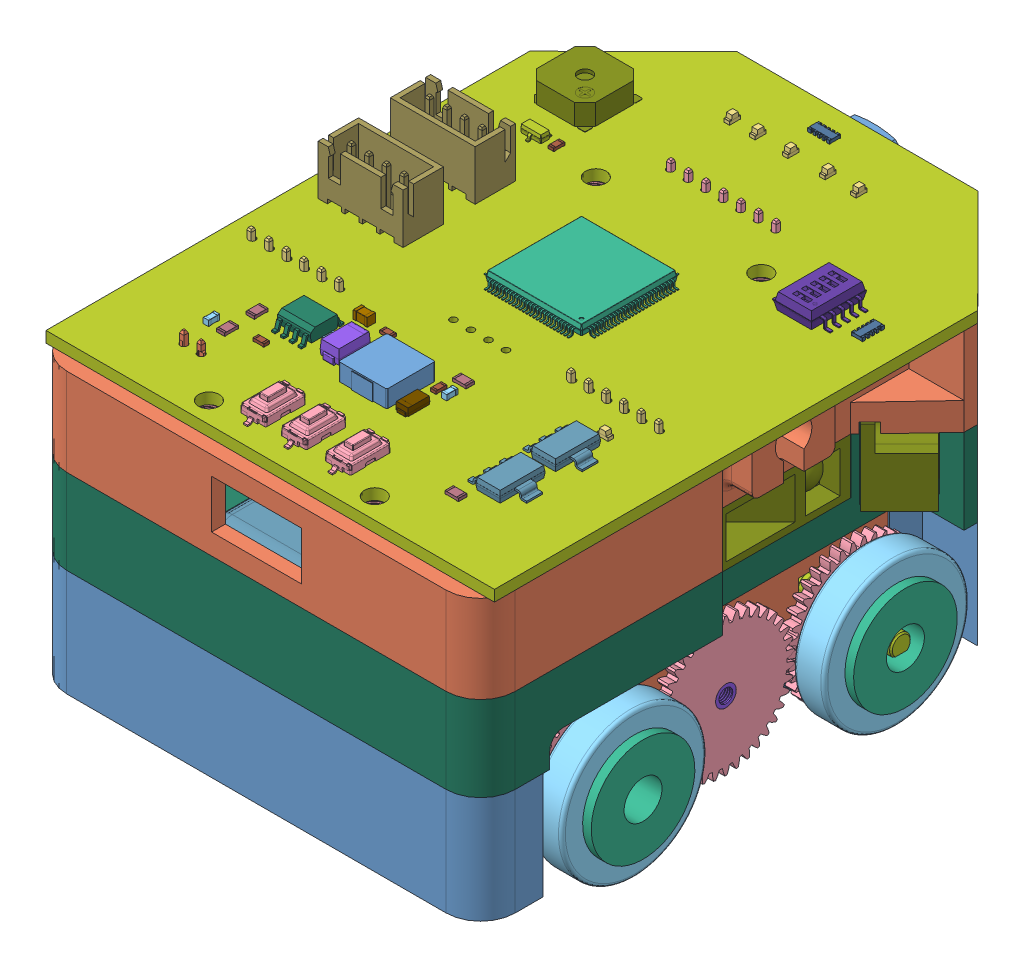
SolidWorks assembly 3.5, configuration Default. Lengths in mm.
Overall size (70.25 55.4 90.5).
225 component instances, 43 part files, 98 mates.
Components (placement in the parent):
- de 3.5-1: de 3.5 [Default] at (21.2951 36.0556 71.295) size (64.97 15.5 87)
- cum banh 3.3-1: cum banh 3.3 [Default] at (54.5824 11.6391 62.8419) x (0 0 1) z (-1 0 0) size (61.54 24.39 40.65)
  - Ga Cum Banh 3.2-1: Ga Cum Banh 3.2 [Default] at (12.9532 31.9165 50.2873) size (60 15.5 15)
  - Bac lot-1: Bac lot [Default] at (-6.0468 31.9165 59.2873) size (9 9 6)
  - spur gear_iso-1: spur gear_iso [ISO - Spur gear 0.5M 38T 20PA 1.5FW ---S38A75H50L3.0N] at (12.9532 31.9165 61.2873) x (0 0 -1) z (0.998859 0.047751 0) size (1.5 19.95 20)
  - Lop banh xe-1: Lop banh xe [Default] at (-6.0468 31.9165 67.7873) x (0 0 -1) z (0.984115 -0.177535 0) size (4.5 21 21)
  - Mam banh xe-1: Mam banh xe [Default] at (-6.0468 31.9165 61.2873) x (-0.608419 -0.793616 0) z (0 0 -1) size (15 15 7)
  - N20 Mini Micro Metall Gear Motor DC 3-6-12V-1: N20 Mini Micro Metall Gear Motor DC 3-6-12V [Default] at (31.9532 31.9165 48.6873) x (0 0 1) z (-1 0 0) size (39.8 12.15 18.58)
  - spur gear_iso-2: spur gear_iso [ISO - Spur gear 0.5M 38T 20PA 1.5FW ---S38A75H50L3.0N] at (31.9532 31.9165 59.7873) x (0 0 1) z (-0.993186 0.116537 0) size (1.5 19.95 20)
  - spur gear_iso-3: spur gear_iso [ISO - Spur gear 0.5M 38T 20PA 1.5FW ---S38A75H50L3.0N] at (-6.0468 31.9165 61.2873) x (0 0 -1) z (1 0 0) size (1.5 19.95 20)
  - Bac lot-2: Bac lot [Default] at (12.9532 31.9165 59.2873) size (9 9 6)
  - Bac lot-3: Bac lot [Default] at (12.9532 31.9165 41.2873) x (0.064602 -0.997911 0) z (0 0 -1) size (9 9 6)
  - Bac lot-4: Bac lot [Default] at (-6.0468 31.9165 41.2873) x (-0.6399 -0.768458 0) z (0 0 -1) size (9 9 6)
  - Tru ren trong-1: Tru ren trong [Default] at (12.9532 31.9165 61.2873) x (0.857173 -0.515029 0) z (0 0 1) size (3 3 20.11)
  - Tru ren trong-2: Tru ren trong [Default] at (-6.0468 31.9165 61.2873) x (-0.86392 -0.50363 0) z (0 0 1) size (3 3 20.11)
  - Lop banh xe-2: Lop banh xe [Default] at (31.9532 31.9165 67.7873) x (0 0 -1) z (-0.996477 0.083863 0) size (4.5 21 21)
  - Mam banh xe 3.3-1: Mam banh xe 3.3 [Default] at (31.9532 31.9165 61.5373) x (-1 0 0) z (0 0 -1) size (15 15 7)
- Bac lot-1: Bac lot [Default] at (47.2951 43.5556 94.795) x (0 0 -1) z (1 0 0) size (9 9 6)
- Tru ren trong-1: Tru ren trong [Default] at (49.2951 43.5556 75.795) x (0 -0.515029 -0.857173) z (1 0 0) size (3 3 20.11)
- Ga Cum Banh 3.2-1: Ga Cum Banh 3.2 [Default] at (38.2951 43.5556 75.795) x (0 0 -1) z (1 0 0) size (60 15.5 15)
- spur gear_iso-1: spur gear_iso [ISO - Spur gear 0.5M 38T 20PA 1.5FW ---S38A75H50L3.0N] at (49.2951 43.5556 94.795) x (-1 0 0) z (0 -0.348165 -0.937433) size (1.5 19.95 20)
- Bac lot-2: Bac lot [Default] at (29.2951 43.5556 94.795) x (0 -0.768458 0.6399) z (-1 0 0) size (9 9 6)
- Mam banh xe-1: Mam banh xe [Default] at (49.2951 43.5556 94.795) x (0 -0.793616 0.608419) z (-1 0 0) size (15 15 7)
- spur gear_iso-2: spur gear_iso [ISO - Spur gear 0.5M 38T 20PA 1.5FW ---S38A75H50L3.0N] at (47.7951 43.5556 56.795) x (1 0 0) z (0 0.906454 -0.422304) size (1.5 19.95 20)
- Lop banh xe-1: Lop banh xe [Default] at (55.7951 43.5556 94.795) x (-1 0 0) z (0 -0.235944 -0.971767) size (4.5 21 21)
- spur gear_iso-3: spur gear_iso [ISO - Spur gear 0.5M 38T 20PA 1.5FW ---S38A75H50L3.0N] at (49.2951 43.5556 75.795) x (-1 0 0) z (0 -0.245069 -0.969506) size (1.5 19.95 20)
- Lop banh xe-2: Lop banh xe [Default] at (55.7951 43.5556 56.795) x (-1 0 0) z (0 -0.354009 -0.935242) size (4.5 21 21)
- Tru ren trong-2: Tru ren trong [Default] at (49.2951 43.5556 94.795) x (0 -0.50363 0.86392) z (1 0 0) size (3 3 20.11)
- Mam banh xe-2: Mam banh xe [Default] at (49.2951 43.5556 56.795) x (0 -0.321252 0.946994) z (-1 0 0) size (15 15 7)
- ga 1-1: ga 1 [Default] at (21.2951 38.5556 41.345) x (0 0 -1) z (1 0 0) size (8.85 13 37.6)
- ga pin-1: ga pin [Default] at (21.2951 50.5556 78.795) x (0 0 -1) z (-1 0 0) size (70 12 15)
- Bac lot-3: Bac lot [Default] at (29.2951 43.5556 75.795) x (0 -0.997911 -0.064602) z (-1 0 0) size (9 9 6)
- N20 Mini Micro Metall Gear Motor DC 3-6-12V-1: N20 Mini Micro Metall Gear Motor DC 3-6-12V [Default] at (36.6951 43.5556 56.795) size (39.8 12.15 18.58)
- GP2Y0A41SK0F-1: GP2Y0A41SK0F [Default] at (21.2951 42.7556 42.295) x (1 0 0) z (0 0 -1) size (29.5 18.9 13.5)
- Bac lot-4: Bac lot [Default] at (47.2951 43.5556 75.795) x (0 0 -1) z (1 0 0) size (9 9 6)
- oc cay m3-1: oc cay m3 [Default] at (8.9051 50.0556 45.895) x (0.952915 0 0.303236) z (-0.303236 0 0.952915) size (5 3.18 5)
- oc cay m3-2: oc cay m3 [Default] at (33.6851 50.0556 45.895) x (-0.705079 0 0.709129) z (-0.709129 0 -0.705079) size (5 3.18 5)
- oc cay m3-3: oc cay m3 [Default] at (38.2951 50.0556 110.295) size (5 3.18 5)
- oc cay m3-4: oc cay m3 [Default] at (4.2951 50.0556 110.295) size (5 3.18 5)
- pin7.4v 2000mAh 30C-1: pin7.4v 2000mAh 30C [Default] at (21.2951 58.5556 113.795) x (1 0 0) z (0 1 0) size (19 73 16)
- pack 1-1: pack 1 [Default] at (21.2951 51.5556 71.295) size (64.97 12.3 87)
- oc cay m3-5: oc cay m3 [Default] at (-6.7254 62.3556 97.7947) size (5 3.18 5)
- oc cay m3-6: oc cay m3 [Default] at (-6.7254 62.3556 109.795) size (5 3.18 5)
- oc cay m3-7: oc cay m3 [Default] at (49.3157 62.3556 97.7947) size (5 3.18 5)
- oc cay m3-8: oc cay m3 [Default] at (49.3157 62.3556 109.795) size (5 3.18 5)
- SHARP GP2Y0A51SK0F.step-1: SHARP GP2Y0A51SK0F.step [Default] at (18.0982 42.1852 55.9924) x (-0.7074 0 0.706814) z (0 1 0) size (27 14.5 13.5)
  - шарп крышка.step-1: шарп крышка.step [Default] at (-12.8819 -17.3225 12.1705) x (1 0 0) z (0 -1 0) size (27 11 12)
  - шарп плата.step-1: шарп плата.step [Default] at (13.6181 -19.3225 25.6705) x (-1 0 0) z (0 -1 0) size (26 13 5.5)
  - 92000A010_Passivated 18-8 Stainless Steel Pan Head Phillips Screws.step-1: 92000A010_Passivated 18-8 Stainless Steel Pan Head Phillips Screws.step [Default] at (11.4181 -22.3225 19.1705) x (1 0 0) z (0 1 0) size (4 4 4.61)
  - 92000A010_Passivated 18-8 Stainless Steel Pan Head Phillips Screws.step-2: 92000A010_Passivated 18-8 Stainless Steel Pan Head Phillips Screws.step [Default] at (-10.1819 -22.3225 14.8705) x (1 0 0) z (0 1 0) size (4 4 4.61)
- SHARP GP2Y0A51SK0F.step-2: SHARP GP2Y0A51SK0F.step [Default] at (25.3665 42.1852 56.8661) x (-0.7074 0 -0.706814) z (0 1 0) size (27 14.5 13.5)
  - шарп крышка.step-1: шарп крышка.step [Default] at (-12.8819 -17.3225 12.1705) x (1 0 0) z (0 -1 0) size (27 11 12)
  - шарп плата.step-1: шарп плата.step [Default] at (13.6181 -19.3225 25.6705) x (-1 0 0) z (0 -1 0) size (26 13 5.5)
  - 92000A010_Passivated 18-8 Stainless Steel Pan Head Phillips Screws.step-1: 92000A010_Passivated 18-8 Stainless Steel Pan Head Phillips Screws.step [Default] at (11.4181 -22.3225 19.1705) x (1 0 0) z (0 1 0) size (4 4 4.61)
  - 92000A010_Passivated 18-8 Stainless Steel Pan Head Phillips Screws.step-2: 92000A010_Passivated 18-8 Stainless Steel Pan Head Phillips Screws.step [Default] at (-10.1819 -22.3225 14.8705) x (1 0 0) z (0 1 0) size (4 4 4.61)
- SHARP GP2Y0A51SK0F.step-3: SHARP GP2Y0A51SK0F.step [Default] at (16.4726 42.1852 64.6239) x (0 0 -1) z (0 1 0) size (27 14.5 13.5)
  - шарп крышка.step-1: шарп крышка.step [Default] at (-12.8819 -17.3225 12.1705) x (1 0 0) z (0 -1 0) size (27 11 12)
  - шарп плата.step-1: шарп плата.step [Default] at (13.6181 -19.3225 25.6705) x (-1 0 0) z (0 -1 0) size (26 13 5.5)
  - 92000A010_Passivated 18-8 Stainless Steel Pan Head Phillips Screws.step-1: 92000A010_Passivated 18-8 Stainless Steel Pan Head Phillips Screws.step [Default] at (11.4181 -22.3225 19.1705) x (1 0 0) z (0 1 0) size (4 4 4.61)
  - 92000A010_Passivated 18-8 Stainless Steel Pan Head Phillips Screws.step-2: 92000A010_Passivated 18-8 Stainless Steel Pan Head Phillips Screws.step [Default] at (-10.1819 -22.3225 14.8705) x (1 0 0) z (0 1 0) size (4 4 4.61)
- SHARP GP2Y0A51SK0F.step-4: SHARP GP2Y0A51SK0F.step [Default] at (26.1177 42.1852 63.3878) x (0 0 1) z (0 1 0) size (27 14.5 13.5)
  - шарп крышка.step-1: шарп крышка.step [Default] at (-12.8819 -17.3225 12.1705) x (1 0 0) z (0 -1 0) size (27 11 12)
  - шарп плата.step-1: шарп плата.step [Default] at (13.6181 -19.3225 25.6705) x (-1 0 0) z (0 -1 0) size (26 13 5.5)
  - 92000A010_Passivated 18-8 Stainless Steel Pan Head Phillips Screws.step-1: 92000A010_Passivated 18-8 Stainless Steel Pan Head Phillips Screws.step [Default] at (11.4181 -22.3225 19.1705) x (1 0 0) z (0 1 0) size (4 4 4.61)
  - 92000A010_Passivated 18-8 Stainless Steel Pan Head Phillips Screws.step-2: 92000A010_Passivated 18-8 Stainless Steel Pan Head Phillips Screws.step [Default] at (-10.1819 -22.3225 14.8705) x (1 0 0) z (0 1 0) size (4 4 4.61)
- Manchester United Logo-1: Manchester United Logo [Varsayılan] at (22.3655 63.775 41.9318) x (-1 0 0) z (0 -1 0) size (25 7.5 25)
- oc cay m3-9: oc cay m3 [Default] at (33.4154 75.0556 110.7741) size (5 3.18 5)
- oc cay m3-10: oc cay m3 [Default] at (9.1749 75.0556 110.7741) size (5 3.18 5)
- oc cay m3-11: oc cay m3 [Default] at (33.4094 75.0556 54.7841) size (5 3.18 5)
- oc cay m3-12: oc cay m3 [Default] at (9.1809 75.0556 54.7841) size (5 3.18 5)
- pack 2-1: pack 2 [Default] at (21.2951 67.8556 71.295) size (64.97 12.7 87)
- schematic (2).step-1: schematic (2).step [Default] at (-158.2053 76.5556 -20.0099) x (1 0 0.000071) z (0 1 0) size (64.97 85.02 16.13)
  - LED_0603_1608Metric.step-1: LED_0603_1608Metric.step [Default] at (188.7822 -57.8002 1.65) x (0 -1 0) z (0 0 1) size (1.6 0.8 1.1)
    - LED_0603_1608Metric-0.step-1: LED_0603_1608Metric-0.step [Default] at origin size (1.6 0.8 1.1)
  - SW_Tactile_SPST_NO_Straight_CK_PTS636Sx25SMTRLFS.step-1: SW_Tactile_SPST_NO_Straight_CK_PTS636Sx25SMTRLFS.step [Default] at (173.4 -127.275 1.65) x (0 1 0) z (0 0 1) size (8 3.7 2.55)
    - PTS636Sx25SMTRLFS.step-1: PTS636Sx25SMTRLFS.step [Default] at origin size (8 3.7 2.55)
  - C_0603_1608Metric.step-1: C_0603_1608Metric.step [Default] at (184.5722 -112.8754 1.65) x (0 1 0) z (0 0 1) size (1.6 0.8 0.8)
    - C_0603_1608Metric-1.step-1: C_0603_1608Metric-1.step [Default] at origin size (1.6 0.8 0.8)
  - LQFP-100_14x14mm_P0.5mm.step-1: LQFP-100_14x14mm_P0.5mm.step [Default] at (179.8 -89 1.65) x (-1 0 0) z (0 0 1) size (16 16 1.5)
    - LQFP_100_14x14mm_P05mm.step-1: LQFP_100_14x14mm_P05mm.step [Default] at origin size (16 16 1.5)
  - SOT-23.step-1: SOT-23.step [Default] at (158.1922 -74.0902 1.65) x (0 -1 0) z (0 0 1) size (2.5 3 1.2)
    - SOT_23.step-1: SOT_23.step [Default] at origin size (2.5 3 1.2)
  - C_0603_1608Metric.step-2: C_0603_1608Metric.step [Default] at (158 -120.8 1.65) x (0 -1 0) z (0 0 1) size (1.6 0.8 0.8)
    - C_0603_1608Metric-1.step-1: C_0603_1608Metric-1.step [Default] at origin size (1.6 0.8 0.8)
  - D_SMA.step-1: D_SMA.step [Default] at (171.575 -115 1.65) x (0 -1 0) z (0 0 1) size (5 2.7 2.22)
    - D_SMA-2.step-1: D_SMA-2.step [Default] at origin size (5 2.7 2.22)
  - C_0805_2012Metric.step-1: C_0805_2012Metric.step [Default] at (168.9622 -109.6002 1.65) size (2 1.25 1.25)
    - C_0805_2012Metric-3.step-1: C_0805_2012Metric-3.step [Default] at origin size (2 1.25 1.25)
  - LED_0603_1608Metric.step-2: LED_0603_1608Metric.step [Default] at (178.88 -57.7875 1.65) x (0 -1 0) z (0 0 1) size (1.6 0.8 1.1)
    - LED_0603_1608Metric-0.step-1: LED_0603_1608Metric-0.step [Default] at origin size (1.6 0.8 1.1)
  - R_Array_Convex_5x0603.step-1: R_Array_Convex_5x0603.step [Default] at (206.8422 -74.5602 1.65) x (-1 0 0) z (0 0 1) size (1.6 3.2 0.5)
    - R_Array_Convex_5x0603-4.step-1: R_Array_Convex_5x0603-4.step [Default] at origin size (1.6 3.2 0.5)
  - R_0603_1608Metric.step-1: R_0603_1608Metric.step [Default] at (161.05 -73.875 1.65) x (0 -1 0) z (0 0 1) size (1.6 0.8 0.45)
    - R_0603_1608Metric-5.step-1: R_0603_1608Metric-5.step [Default] at origin size (1.6 0.8 0.45)
  - R_0603_1608Metric.step-2: R_0603_1608Metric.step [Default] at (155.05 -78.75 1.65) x (0 -1 0) z (0 0 1) size (1.6 0.8 0.45)
    - R_0603_1608Metric-5.step-1: R_0603_1608Metric-5.step [Default] at origin size (1.6 0.8 0.45)
  - R_0603_1608Metric.step-3: R_0603_1608Metric.step [Default] at (157.65 -78.75 1.65) x (0 -1 0) z (0 0 1) size (1.6 0.8 0.45)
    - R_0603_1608Metric-5.step-1: R_0603_1608Metric-5.step [Default] at origin size (1.6 0.8 0.45)
  - JST - XH - Thru (V) - 4Pin - 2.54mm.step-1: JST - XH - Thru (V) - 4Pin - 2.54mm.step [Default] at (156.4 -95.1037 1.65) size (12.29 5.84 10.21)
    - JST - XH - Thru - 4Pin - 2.54mm.step-1: JST - XH - Thru - 4Pin - 2.54mm.step [Default] at origin size (12.29 5.84 10.21)
  - C_0603_1608Metric.step-3: C_0603_1608Metric.step [Default] at (169.0522 -114.6252 1.65) x (0 1 0) z (0 0 1) size (1.6 0.8 0.8)
    - C_0603_1608Metric-1.step-1: C_0603_1608Metric-1.step [Default] at origin size (1.6 0.8 0.8)
  - LED_0603_1608Metric.step-3: LED_0603_1608Metric.step [Default] at (184.2422 -57.7602 1.65) x (0 -1 0) z (0 0 1) size (1.6 0.8 1.1)
    - LED_0603_1608Metric-0.step-1: LED_0603_1608Metric-0.step [Default] at origin size (1.6 0.8 1.1)
  - R_0805_2012Metric.step-1: R_0805_2012Metric.step [Default] at (160.2 -116.4 1.65) x (0 1 0) z (0 0 1) size (2 1.2 0.45)
    - R_0805_2012Metric-6.step-1: R_0805_2012Metric-6.step [Default] at origin size (2 1.2 0.45)
  - JST - XH - Thru (V) - 4Pin - 2.54mm.step-2: JST - XH - Thru (V) - 4Pin - 2.54mm.step [Default] at (156.19 -83.5908 1.65) x (-1 0 0) z (0 0 1) size (12.29 5.84 10.21)
    - JST - XH - Thru - 4Pin - 2.54mm.step-1: JST - XH - Thru - 4Pin - 2.54mm.step [Default] at origin size (12.29 5.84 10.21)
  - R_0805_2012Metric.step-2: R_0805_2012Metric.step [Default] at (183.8822 -110.1902 1.65) x (-1 0 0) z (0 0 1) size (2 1.2 0.45)
    - R_0805_2012Metric-6.step-1: R_0805_2012Metric-6.step [Default] at origin size (2 1.2 0.45)
  - SOT-223.step-1: SOT-223.step [Default] at (200.0875 -119.57 1.65) size (7 6.5 1.7)
    - SOT_223.step-1: SOT_223.step [Default] at origin size (7 6.5 1.7)
  - SOT-223.step-2: SOT-223.step [Default] at (200.1422 -111.6002 1.65) size (7 6.5 1.7)
    - SOT_223.step-1: SOT_223.step [Default] at origin size (7 6.5 1.7)
  - R_0603_1608Metric.step-4: R_0603_1608Metric.step [Default] at (172.4222 -109.6502 1.65) size (1.6 0.8 0.45)
    - R_0603_1608Metric-5.step-1: R_0603_1608Metric-5.step [Default] at origin size (1.6 0.8 0.45)
  - LED_0603_1608Metric.step-4: LED_0603_1608Metric.step [Default] at (174.1622 -57.8202 1.65) x (0 -1 0) z (0 0 1) size (1.6 0.8 1.1)
    - LED_0603_1608Metric-0.step-1: LED_0603_1608Metric-0.step [Default] at origin size (1.6 0.8 1.1)
  - R_0805_2012Metric.step-3: R_0805_2012Metric.step [Default] at (160.2 -120.6875 1.65) x (0 1 0) z (0 0 1) size (2 1.2 0.45)
    - R_0805_2012Metric-6.step-1: R_0805_2012Metric-6.step [Default] at origin size (2 1.2 0.45)
  - R_Array_Convex_5x0603.step-2: R_Array_Convex_5x0603.step [Default] at (178.8922 -52.9602 1.65) x (0 1 0) z (0 0 1) size (1.6 3.2 0.5)
    - R_Array_Convex_5x0603-4.step-1: R_Array_Convex_5x0603-4.step [Default] at origin size (1.6 3.2 0.5)
  - SW_Tactile_SPST_NO_Straight_CK_PTS636Sx25SMTRLFS.step-2: SW_Tactile_SPST_NO_Straight_CK_PTS636Sx25SMTRLFS.step [Default] at (179.2 -127.2 1.65) x (0 1 0) z (0 0 1) size (8 3.7 2.55)
    - PTS636Sx25SMTRLFS.step-1: PTS636Sx25SMTRLFS.step [Default] at origin size (8 3.7 2.55)
  - SO-8_narrow_simple.step-1: SO-8_narrow_simple.step [Default] at (165.7508 -114.6 1.65) x (-1 0 0) z (0 0 1) size (4.8 6.2 2)
    - ASSEMBLY.step-1: ASSEMBLY.step [Default] at origin size (4.8 6.2 2)
  - SW_Tactile_SPST_NO_Straight_CK_PTS636Sx25SMTRLFS.step-3: SW_Tactile_SPST_NO_Straight_CK_PTS636Sx25SMTRLFS.step [Default] at (185.6 -127.2 1.65) x (0 1 0) z (0 0 1) size (8 3.7 2.55)
    - PTS636Sx25SMTRLFS.step-1: PTS636Sx25SMTRLFS.step [Default] at origin size (8 3.7 2.55)
  - LED_0603_1608Metric.step-5: LED_0603_1608Metric.step [Default] at (200.9422 -106.7002 1.65) x (-1 0 0) z (0 0 1) size (1.6 0.8 1.1)
    - LED_0603_1608Metric-0.step-1: LED_0603_1608Metric-0.step [Default] at origin size (1.6 0.8 1.1)
  - LED_0603_1608Metric.step-6: LED_0603_1608Metric.step [Default] at (170.4722 -57.8302 1.65) x (0 -1 0) z (0 0 1) size (1.6 0.8 1.1)
    - LED_0603_1608Metric-0.step-1: LED_0603_1608Metric-0.step [Default] at origin size (1.6 0.8 1.1)
  - GSC8530YA-16R2700.step-1: GSC8530YA-16R2700.step [Default] at (157.0222 -65.7202 1.65) x (-1 0 0) z (0 1 0) size (8.55 3.15 8.5)
    - GSC8530YA-16R2700-7.step-1: GSC8530YA-16R2700-7.step [Default] at origin size (8.55 3.15 8.5)
  - SW_DIP_SPSTx05_Slide_KingTek_DSHP05TS_W7.62mm_P1.27mm.step-1: SW_DIP_SPSTx05_Slide_KingTek_DSHP05TS_W7.62mm_P1.27mm.step [Default] at (200.1022 -74.7302 1.65) x (-1 0 0) z (0 0 1) size (8.35 7.95 2.38)
    - SW_DIP_SPSTx05_Slide_KingTek_DSHP05TS_W762mm_P127mm.step-1: SW_DIP_SPSTx05_Slide_KingTek_DSHP05TS_W762mm_P127mm.step [Default] at origin size (8.35 7.95 2.38)
  - R_0603_1608Metric.step-5: R_0603_1608Metric.step [Default] at (182.9722 -112.8652 1.65) x (0 1 0) z (0 0 1) size (1.6 0.8 0.45)
    - R_0603_1608Metric-5.step-1: R_0603_1608Metric-5.step [Default] at origin size (1.6 0.8 0.45)
  - R_0805_2012Metric.step-4: R_0805_2012Metric.step [Default] at (197.4675 -124.865 1.65) size (2 1.2 0.45)
    - R_0805_2012Metric-6.step-1: R_0805_2012Metric-6.step [Default] at origin size (2 1.2 0.45)
  - CP_EIA-3216-10_Kemet-I.step-1: CP_EIA-3216-10_Kemet-I.step [Default] at (183.3922 -117.0302 1.65) x (0 1 0) z (0 0 1) size (3.4 1.8 1.2)
    - CP_EIA_3216_10_Kemet_I.step-1: CP_EIA_3216_10_Kemet_I.step [Default] at origin size (3.4 1.8 1.2)
  - Inductor_7x7x2.5.step-1: Inductor_7x7x2.5.step [Default] at (178.1322 -115.5302 1.65) x (1 0 0) z (0 -1 0) size (7 2.6 7.2)
    - Inductor_7x7x2.5-8.step-1: Inductor_7x7x2.5-8.step [Default] at origin size (7 2.6 7.2)
  - R_0603_1608Metric.step-6: R_0603_1608Metric.step [Default] at (164.2 -119.8 1.65) x (-1 0 0) z (0 0 1) size (1.6 0.8 0.45)
    - R_0603_1608Metric-5.step-1: R_0603_1608Metric-5.step [Default] at origin size (1.6 0.8 0.45)
  - C_0603_1608Metric.step-4: C_0603_1608Metric.step [Default] at (195.3522 -91.7102 -0.05) x (1 0 0) z (0 0 -1) size (1.6 0.8 0.8)
    - C_0603_1608Metric-1.step-1: C_0603_1608Metric-1.step [Default] at origin size (1.6 0.8 0.8)
  - C_0603_1608Metric.step-5: C_0603_1608Metric.step [Default] at (180.3022 -85.9102 -0.05) x (-1 0 0) z (0 0 -1) size (1.6 0.8 0.8)
    - C_0603_1608Metric-1.step-1: C_0603_1608Metric-1.step [Default] at origin size (1.6 0.8 0.8)
  - C_0603_1608Metric.step-6: C_0603_1608Metric.step [Default] at (183.6572 -94.2302 -0.05) x (-1 0 0) z (0 0 -1) size (1.6 0.8 0.8)
    - C_0603_1608Metric-1.step-1: C_0603_1608Metric-1.step [Default] at origin size (1.6 0.8 0.8)
  - B2B-XH-A_LF__SN_.step-1: B2B-XH-A_LF__SN_.step [Default] at (159.9422 -124.9552 -0.05) x (-1 0 0) z (0 -1 0) size (7.4 10.4 5.75)
    - B2B-XH-A(LF)(SN).step-1: B2B-XH-A(LF)(SN).step [Default] at origin size (7.4 10.4 5.75)
  - R_0603_1608Metric.step-7: R_0603_1608Metric.step [Default] at (179.7 -125.6 -0.05) x (-1 0 0) z (0 0 -1) size (1.6 0.8 0.45)
    - R_0603_1608Metric-5.step-1: R_0603_1608Metric-5.step [Default] at origin size (1.6 0.8 0.45)
  - JST - XH - Thru (V) - 6Pin - 2.54mm.step-1: JST - XH - Thru (V) - 6Pin - 2.54mm.step [Default] at (197.6322 -101.9902 -0.05) x (1 0 0) z (0 0 -1) size (17.37 5.84 10.21)
    - JST - XH - Thru - 6Pin - 2.54mm.step-1: JST - XH - Thru - 6Pin - 2.54mm.step [Default] at origin size (17.37 5.84 10.21)
  - CP_EIA-3216-10_Kemet-I.step-2: CP_EIA-3216-10_Kemet-I.step [Default] at (201.5522 -117.3902 -0.05) x (1 0 0) z (0 0 -1) size (3.4 1.8 1.2)
    - CP_EIA_3216_10_Kemet_I.step-1: CP_EIA_3216_10_Kemet_I.step [Default] at origin size (3.4 1.8 1.2)
  - CP_EIA-3216-10_Kemet-I.step-3: CP_EIA-3216-10_Kemet-I.step [Default] at (177.2197 -105.6402 -0.05) x (-1 0 0) z (0 0 -1) size (3.4 1.8 1.2)
    - CP_EIA_3216_10_Kemet_I.step-1: CP_EIA_3216_10_Kemet_I.step [Default] at origin size (3.4 1.8 1.2)
  - R_0603_1608Metric.step-8: R_0603_1608Metric.step [Default] at (174.2 -125.475 -0.05) x (-1 0 0) z (0 0 -1) size (1.6 0.8 0.45)
    - R_0603_1608Metric-5.step-1: R_0603_1608Metric-5.step [Default] at origin size (1.6 0.8 0.45)
  - C_0603_1608Metric.step-7: C_0603_1608Metric.step [Default] at (183.6972 -92.4602 -0.05) x (-1 0 0) z (0 0 -1) size (1.6 0.8 0.8)
    - C_0603_1608Metric-1.step-1: C_0603_1608Metric-1.step [Default] at origin size (1.6 0.8 0.8)
  - CP_EIA-3216-10_Kemet-I.step-4: CP_EIA-3216-10_Kemet-I.step [Default] at (171.2722 -117.1002 -0.05) x (0 -1 0) z (0 0 -1) size (3.4 1.8 1.2)
    - CP_EIA_3216_10_Kemet_I.step-1: CP_EIA_3216_10_Kemet_I.step [Default] at origin size (3.4 1.8 1.2)
  - C_0603_1608Metric.step-8: C_0603_1608Metric.step [Default] at (184.8 -125.6 -0.05) x (1 0 0) z (0 0 -1) size (1.6 0.8 0.8)
    - C_0603_1608Metric-1.step-1: C_0603_1608Metric-1.step [Default] at origin size (1.6 0.8 0.8)
  - JST - XH - Thru (V) - 6Pin - 2.54mm.step-2: JST - XH - Thru (V) - 6Pin - 2.54mm.step [Default] at (156.6722 -107.3602 -0.05) x (1 0 0) z (0 0 -1) size (17.37 5.84 10.21)
    - JST - XH - Thru - 6Pin - 2.54mm.step-1: JST - XH - Thru - 6Pin - 2.54mm.step [Default] at origin size (17.37 5.84 10.21)
  - C_0603_1608Metric.step-9: C_0603_1608Metric.step [Default] at (177.5197 -107.4902 -0.05) x (-1 0 0) z (0 0 -1) size (1.6 0.8 0.8)
    - C_0603_1608Metric-1.step-1: C_0603_1608Metric-1.step [Default] at origin size (1.6 0.8 0.8)
  - JST - XH - Thru (V) - 7Pin - 2.54mm.step-1: JST - XH - Thru (V) - 7Pin - 2.54mm.step [Default] at (179.7522 -68.3802 -0.05) x (1 0 0) z (0 0 -1) size (19.91 5.84 10.21)
    - JST - XH - Thru - 7Pin - 2.54mm.step-1: JST - XH - Thru - 7Pin - 2.54mm.step [Default] at origin size (19.91 5.84 10.21)
  - C_0603_1608Metric.step-10: C_0603_1608Metric.step [Default] at (180.31 -87.58 -0.05) x (-1 0 0) z (0 0 -1) size (1.6 0.8 0.8)
    - C_0603_1608Metric-1.step-1: C_0603_1608Metric-1.step [Default] at origin size (1.6 0.8 0.8)
  - C_0603_1608Metric.step-11: C_0603_1608Metric.step [Default] at (183.6272 -88.9602 -0.05) x (-1 0 0) z (0 0 -1) size (1.6 0.8 0.8)
    - C_0603_1608Metric-1.step-1: C_0603_1608Metric-1.step [Default] at origin size (1.6 0.8 0.8)
  - CP_EIA-3216-10_Kemet-I.step-5: CP_EIA-3216-10_Kemet-I.step [Default] at (201.5422 -113.8002 -0.05) x (1 0 0) z (0 0 -1) size (3.4 1.8 1.2)
    - CP_EIA_3216_10_Kemet_I.step-1: CP_EIA_3216_10_Kemet_I.step [Default] at origin size (3.4 1.8 1.2)
  - R_0603_1608Metric.step-9: R_0603_1608Metric.step [Default] at (160.18 -91.9945 -0.05) x (0 1 0) z (0 0 -1) size (1.6 0.8 0.45)
    - R_0603_1608Metric-5.step-1: R_0603_1608Metric-5.step [Default] at origin size (1.6 0.8 0.45)
  - C_0603_1608Metric.step-12: C_0603_1608Metric.step [Default] at (183.5822 -85.8802 -0.05) x (1 0 0) z (0 0 -1) size (1.6 0.8 0.8)
    - C_0603_1608Metric-1.step-1: C_0603_1608Metric-1.step [Default] at origin size (1.6 0.8 0.8)
  - C_0603_1608Metric.step-13: C_0603_1608Metric.step [Default] at (175.4 -92.9 -0.05) x (1 0 0) z (0 0 -1) size (1.6 0.8 0.8)
    - C_0603_1608Metric-1.step-1: C_0603_1608Metric-1.step [Default] at origin size (1.6 0.8 0.8)
  - C_0603_1608Metric.step-14: C_0603_1608Metric.step [Default] at (195.4222 -86.5502 -0.05) x (1 0 0) z (0 0 -1) size (1.6 0.8 0.8)
    - C_0603_1608Metric-1.step-1: C_0603_1608Metric-1.step [Default] at origin size (1.6 0.8 0.8)
  - C_0603_1608Metric.step-15: C_0603_1608Metric.step [Default] at (183.6122 -84.1702 -0.05) x (1 0 0) z (0 0 -1) size (1.6 0.8 0.8)
    - C_0603_1608Metric-1.step-1: C_0603_1608Metric-1.step [Default] at origin size (1.6 0.8 0.8)
  - R_0603_1608Metric.step-10: R_0603_1608Metric.step [Default] at (200.5422 -109.4502 -0.05) x (-1 0 0) z (0 0 -1) size (1.6 0.8 0.45)
    - R_0603_1608Metric-5.step-1: R_0603_1608Metric-5.step [Default] at origin size (1.6 0.8 0.45)
  - Crystal_SMD_3225-4Pin_3.2x2.5mm.step-1: Crystal_SMD_3225-4Pin_3.2x2.5mm.step [Default] at (195.4222 -89.2002 -0.05) x (1 0 0) z (0 0 -1) size (3.2 2.5 0.64)
    - Crystal_SMD_3225-4Pin_3.2x2.5mm-9.step-1: Crystal_SMD_3225-4Pin_3.2x2.5mm-9.step [Default] at origin size (3.2 2.5 0.64)
  - C_0603_1608Metric.step-16: C_0603_1608Metric.step [Default] at (183.6 -82.6 -0.05) x (-1 0 0) z (0 0 -1) size (1.6 0.8 0.8)
    - C_0603_1608Metric-1.step-1: C_0603_1608Metric-1.step [Default] at origin size (1.6 0.8 0.8)
  - R_0603_1608Metric.step-11: R_0603_1608Metric.step [Default] at (157.68 -91.9445 -0.05) x (0 -1 0) z (0 0 -1) size (1.6 0.8 0.45)
    - R_0603_1608Metric-5.step-1: R_0603_1608Metric-5.step [Default] at origin size (1.6 0.8 0.45)
  - C_0603_1608Metric.step-17: C_0603_1608Metric.step [Default] at (179.7 -128.5 -0.05) x (-1 0 0) z (0 0 -1) size (1.6 0.8 0.8)
    - C_0603_1608Metric-1.step-1: C_0603_1608Metric-1.step [Default] at origin size (1.6 0.8 0.8)
  - R_0603_1608Metric.step-12: R_0603_1608Metric.step [Default] at (183.7 -97.3 -0.05) x (-1 0 0) z (0 0 -1) size (1.6 0.8 0.45)
    - R_0603_1608Metric-5.step-1: R_0603_1608Metric-5.step [Default] at origin size (1.6 0.8 0.45)
  - C_0603_1608Metric.step-18: C_0603_1608Metric.step [Default] at (174.2 -128.275 -0.05) x (-1 0 0) z (0 0 -1) size (1.6 0.8 0.8)
    - C_0603_1608Metric-1.step-1: C_0603_1608Metric-1.step [Default] at origin size (1.6 0.8 0.8)
  - C_0603_1608Metric.step-19: C_0603_1608Metric.step [Default] at (183.6 -90.7 -0.05) x (-1 0 0) z (0 0 -1) size (1.6 0.8 0.8)
    - C_0603_1608Metric-1.step-1: C_0603_1608Metric-1.step [Default] at origin size (1.6 0.8 0.8)
  - CP_EIA-3216-10_Kemet-I.step-6: CP_EIA-3216-10_Kemet-I.step [Default] at (201.5422 -111.5502 -0.05) x (1 0 0) z (0 0 -1) size (3.4 1.8 1.2)
    - CP_EIA_3216_10_Kemet_I.step-1: CP_EIA_3216_10_Kemet_I.step [Default] at origin size (3.4 1.8 1.2)
  - C_0603_1608Metric.step-20: C_0603_1608Metric.step [Default] at (152.48 -91.8945 -0.05) x (0 1 0) z (0 0 -1) size (1.6 0.8 0.8)
    - C_0603_1608Metric-1.step-1: C_0603_1608Metric-1.step [Default] at origin size (1.6 0.8 0.8)
  - C_0603_1608Metric.step-21: C_0603_1608Metric.step [Default] at (176.7 -85.4 -0.05) x (1 0 0) z (0 0 -1) size (1.6 0.8 0.8)
    - C_0603_1608Metric-1.step-1: C_0603_1608Metric-1.step [Default] at origin size (1.6 0.8 0.8)
  - C_0603_1608Metric.step-22: C_0603_1608Metric.step [Default] at (176.7 -83.7 -0.05) x (1 0 0) z (0 0 -1) size (1.6 0.8 0.8)
    - C_0603_1608Metric-1.step-1: C_0603_1608Metric-1.step [Default] at origin size (1.6 0.8 0.8)
  - C_0603_1608Metric.step-23: C_0603_1608Metric.step [Default] at (175.4 -94.5 -0.05) x (1 0 0) z (0 0 -1) size (1.6 0.8 0.8)
    - C_0603_1608Metric-1.step-1: C_0603_1608Metric-1.step [Default] at origin size (1.6 0.8 0.8)
  - CP_EIA-3216-10_Kemet-I.step-7: CP_EIA-3216-10_Kemet-I.step [Default] at (201.5375 -122.02 -0.05) x (1 0 0) z (0 0 -1) size (3.4 1.8 1.2)
    - CP_EIA_3216_10_Kemet_I.step-1: CP_EIA_3216_10_Kemet_I.step [Default] at origin size (3.4 1.8 1.2)
  - C_0603_1608Metric.step-24: C_0603_1608Metric.step [Default] at (173.1722 -116.6002 -0.05) x (0 -1 0) z (0 0 -1) size (1.6 0.8 0.8)
    - C_0603_1608Metric-1.step-1: C_0603_1608Metric-1.step [Default] at origin size (1.6 0.8 0.8)
  - SSOP-24_5.3x8.2mm_P0.65mm.step-1: SSOP-24_5.3x8.2mm_P0.65mm.step [Default] at (178.875 -116.225 -0.05) x (0 1 0) z (0 0 -1) size (7.8 8.2 2.1)
    - SSOP_24_53x82mm_P065mm.step-1: SSOP_24_53x82mm_P065mm.step [Default] at origin size (7.8 8.2 2.1)
  - schematic_PCB.step-1: schematic_PCB.step [Default] at origin size (64.97 85.02 1.6)
Mates (geometry in assembly coordinates):
- Coincident1: coincident anti-aligned: plane of Ga Cum Banh 3.2-1 through (30.7951 43.5556 75.795) normal (-1 0 0); plane of Bac lot-2 through (30.7951 41.2503 96.7147) normal (1 0 0)
- Coincident2: coincident anti-aligned: plane of Ga Cum Banh 3.2-1 through (45.7951 49.5556 75.795) normal (0 -1 0); plane of N20 Mini Micro Metall Gear Motor DC 3-6-12V-1 through (40.7951 49.5556 51.795) normal (0 1 0)
- Concentric1: concentric anti-aligned: cylinder of Ga Cum Banh 3.2-1 through (45.7951 43.5556 75.795) axis (-1 0 0) radius 3.15; cylinder of Bac lot-4 through (47.2951 43.5556 75.795) axis (1 0 0) radius 3
- Concentric2: concentric anti-aligned: cylinder of Ga Cum Banh 3.2-1 through (45.7951 43.5556 94.795) axis (-1 0 0) radius 3.15; cylinder of spur gear_iso-1 through (-0.7049 43.5556 94.795) axis (1 0 0) radius 1.5
- Concentric3: concentric anti-aligned: cylinder of N20 Mini Micro Metall Gear Motor DC 3-6-12V-1 through (55.6951 43.5556 56.795) axis (1 0 0) radius 1.5; cylinder of spur gear_iso-2 through (97.7952 43.5556 56.795) axis (-1 0 0) radius 1.5
- Concentric4: concentric anti-aligned: cylinder of Ga Cum Banh 3.2-1 through (45.7951 43.5556 75.795) axis (-1 0 0) radius 3.15; cylinder of spur gear_iso-3 through (-0.7049 43.5556 75.795) axis (1 0 0) radius 1.5
- Coincident3: coincident aligned: plane of spur gear_iso-1 through (47.7951 43.5556 94.795) normal (-1 0 0); plane of spur gear_iso-3 through (47.7951 43.5556 75.795) normal (-1 0 0)
- Coincident4: coincident aligned: plane of spur gear_iso-2 through (47.7951 43.5556 56.795) normal (-1 0 0); plane of spur gear_iso-3 through (47.7951 43.5556 75.795) normal (-1 0 0)
- Concentric5: concentric aligned: cylinder of Ga Cum Banh 3.2-1 through (45.7951 43.5556 94.795) axis (-1 0 0) radius 3.15; cylinder of Bac lot-2 through (29.2951 43.5556 94.795) axis (-1 0 0) radius 3
- Concentric6: concentric anti-aligned: cylinder of Bac lot-1 through (47.2951 43.5556 94.795) axis (1 0 0) radius 3; cylinder of Ga Cum Banh 3.2-1 through (45.7951 43.5556 94.795) axis (-1 0 0) radius 3.15
- Width1: width anti-aligned: plane of N20 Mini Micro Metall Gear Motor DC 3-6-12V-1 through (36.6951 37.5556 51.795) normal (0 0 -1); plane of Ga Cum Banh 3.2-1 through (36.6951 49.5556 61.795) normal (0 0 1); plane of N20 Mini Micro Metall Gear Motor DC 3-6-12V-1 through (45.7951 43.5556 51.795) normal (0 0 1); plane of Ga Cum Banh 3.2-1 through (45.7951 43.5556 61.795) normal (0 0 -1)
- Coincident5: coincident anti-aligned: plane of Bac lot-1 through (45.7951 43.5556 91.795) normal (-1 0 0); plane of Ga Cum Banh 3.2-1 through (45.7951 43.5556 75.795) normal (1 0 0)
- Coincident6: coincident anti-aligned: plane of Mam banh xe-1 through (50.5451 37.6035 99.3582) normal (1 0 0); plane of Lop banh xe-1 through (50.5451 53.7592 92.3176) normal (-1 0 0)
- Concentric7: concentric anti-aligned: cylinder of N20 Mini Micro Metall Gear Motor DC 3-6-12V-1 through (55.6951 43.5556 56.795) axis (1 0 0) radius 1.5; cylinder of Mam banh xe-2 through (49.2951 43.5556 56.795) axis (-1 0 0) radius 2.75
- Concentric8: concentric anti-aligned: cylinder of Lop banh xe-2 through (55.7951 43.5556 56.795) axis (1 0 0) radius 5.5; cylinder of Mam banh xe-2 through (49.2951 43.5556 56.795) axis (-1 0 0) radius 5.5
- Distance1: distance = 0.5 mm anti-aligned: plane of spur gear_iso-3 through (47.7951 43.5556 75.795) normal (-1 0 0); plane of Bac lot-4 through (47.2951 43.5556 71.295) normal (1 0 0)
- Concentric9: concentric aligned: cylinder of Tru ren trong-1 through (49.2951 43.5556 75.795) axis (1 0 0) radius 1.5; cylinder of spur gear_iso-3 through (-0.7049 43.5556 75.795) axis (1 0 0) radius 1.5
- Coincident8: coincident anti-aligned: plane of Ga Cum Banh 3.2-1 through (30.7951 43.5556 75.795) normal (-1 0 0); plane of Bac lot-3 through (30.7951 40.5619 75.6012) normal (1 0 0)
- Concentric10: concentric anti-aligned: cylinder of Bac lot-2 through (29.2951 43.5556 94.795) axis (-1 0 0) radius 1.65; cylinder of Tru ren trong-2 through (49.2951 43.5556 94.795) axis (1 0 0) radius 1.5
- Concentric11: concentric anti-aligned: cylinder of Mam banh xe-1 through (49.2951 43.5556 94.795) axis (-1 0 0) radius 5.5; cylinder of Lop banh xe-1 through (55.7951 43.5556 94.795) axis (1 0 0) radius 5.5
- Coincident9: coincident anti-aligned: plane of Ga Cum Banh 3.2-1 through (45.7951 43.5556 75.795) normal (1 0 0); plane of Bac lot-4 through (45.7951 43.5556 72.795) normal (-1 0 0)
- Concentric12: concentric aligned: cylinder of Ga Cum Banh 3.2-1 through (45.7951 43.5556 75.795) axis (-1 0 0) radius 3.15; cylinder of Bac lot-3 through (29.2951 43.5556 75.795) axis (-1 0 0) radius 3
- Distance2: distance = 0.5 mm anti-aligned: plane of spur gear_iso-2 through (47.7951 43.5556 56.795) normal (-1 0 0); plane of N20 Mini Micro Metall Gear Motor DC 3-6-12V-1 through (47.2951 41.0556 54.295) normal (1 0 0)
- Coincident10: coincident anti-aligned: plane of Lop banh xe-2 through (50.5451 53.3757 53.0779) normal (-1 0 0); plane of Mam banh xe-2 through (50.5451 41.1462 63.8975) normal (1 0 0)
- Concentric13: concentric anti-aligned: cylinder of Mam banh xe-1 through (49.2951 43.5556 94.795) axis (-1 0 0) radius 1.65; circle of Tru ren trong-2
- Coincident11: coincident anti-aligned: plane of spur gear_iso-1 through (49.2951 43.5556 94.795) normal (1 0 0); plane of Mam banh xe-1 through (49.2951 42.2462 95.7989) normal (-1 0 0)
- Coincident12: coincident aligned: plane of Bac lot-2 through (29.2951 40.0976 97.6746) normal (-1 0 0); plane of Tru ren trong-2 through (29.2951 42.8002 96.0909) normal (-1 0 0)
- Coincident13: coincident aligned: plane of Tru ren trong-1 through (49.2951 43.0406 74.9379) normal (1 0 0); plane of spur gear_iso-3 through (49.2951 43.5556 75.795) normal (1 0 0)
- Coincident14: coincident anti-aligned: plane of de 3.5-1 through (21.2951 38.5556 71.295) normal (0 1 0); plane of cum banh 3.3-1/Ga Cum Banh 3.2-1 through (-3.2049 38.5556 75.795) normal (0 -1 0)
- Coincident15: coincident anti-aligned: plane of de 3.5-1 through (21.2951 38.5556 71.295) normal (0 1 0); plane of Ga Cum Banh 3.2-1 through (45.7951 38.5556 75.795) normal (0 -1 0)
- Width2: width anti-aligned: plane of Ga Cum Banh 3.2-1 through (45.7951 43.5556 45.795) normal (0 0 -1); plane of de 3.5-1 through (45.7951 43.5556 105.795) normal (0 0 1); plane of Ga Cum Banh 3.2-1 through (36.4951 51.5556 45.495) normal (0 0 1); plane of de 3.5-1 through (40.0951 51.5556 106.095) normal (0 0 -1)
- Width3: width anti-aligned: plane of Ga Cum Banh 3.2-1 through (36.7951 43.5556 75.795) normal (-1 0 0); plane of de 3.5-1 through (39.7951 43.5556 75.795) normal (1 0 0); plane of Ga Cum Banh 3.2-1 through (36.4951 51.5556 106.095) normal (1 0 0); plane of de 3.5-1 through (40.0951 51.5556 102.995) normal (-1 0 0)
- Width4: width aligned: plane of cum banh 3.3-1/Ga Cum Banh 3.2-1 through (-3.2049 43.5556 105.795) normal (0 0 1); plane of de 3.5-1 through (-3.2049 43.5556 45.795) normal (0 0 -1); plane of cum banh 3.3-1/Ga Cum Banh 3.2-1 through (6.0951 51.5556 45.495) normal (0 0 1); plane of de 3.5-1 through (2.4951 51.5556 106.095) normal (0 0 -1)
- Width5: width anti-aligned: plane of cum banh 3.3-1/Ga Cum Banh 3.2-1 through (2.7951 43.5556 75.795) normal (-1 0 0); plane of de 3.5-1 through (5.7951 43.5556 75.795) normal (1 0 0); plane of cum banh 3.3-1/Ga Cum Banh 3.2-1 through (2.4951 51.5556 102.995) normal (1 0 0); plane of de 3.5-1 through (6.0951 51.5556 106.095) normal (-1 0 0)
- Width6: width anti-aligned: plane of ga 1-1 through (2.4951 38.5556 40.645) normal (-1 0 0); plane of de 3.5-1 through (40.0951 38.5556 40.645) normal (1 0 0); plane of ga 1-1 through (2.2951 51.5556 38.795) normal (1 0 0); plane of de 3.5-1 through (40.2951 51.5556 38.795) normal (-1 0 0)
- Width7: width anti-aligned: plane of GP2Y0A41SK0F-1 through (36.0451 46.9556 42.295) normal (1 0 0); plane of de 3.5-1 through (6.5451 38.5556 42.295) normal (-1 0 0); plane of GP2Y0A41SK0F-1 through (37.2577 51.5556 28.795) normal (-1 0 0); plane of de 3.5-1 through (5.3326 51.5556 28.795) normal (1 0 0)
- Coincident16: coincident anti-aligned: plane of de 3.5-1 through (21.2951 38.5556 71.295) normal (0 1 0); plane of GP2Y0A41SK0F-1 through (36.0451 38.5556 42.295) normal (0 -1 0)
- Width8: width anti-aligned: plane of GP2Y0A41SK0F-1 through (21.2951 37.4056 35.095) normal (0 0 -1); plane of de 3.5-1 through (11.0451 42.7556 42.295) normal (0 0 1); plane of GP2Y0A41SK0F-1 through (36.2451 46.0556 34.895) normal (0 0 1); plane of de 3.5-1 through (6.3451 46.0556 42.495) normal (0 0 -1)
- Width9: width aligned: plane of ga 1-1 through (40.0951 38.5556 39.045) normal (0 0 -1); plane of de 3.5-1 through (40.0951 38.5556 40.645) normal (0 0 1); plane of ga 1-1 through (40.2951 51.5556 40.895) normal (0 0 -1); plane of de 3.5-1 through (37.2577 51.5556 38.795) normal (0 0 1)
- Coincident17: coincident aligned: plane of de 3.5-1 through (21.2951 51.5556 71.295) normal (0 1 0); plane of ga 1-1 through (40.2951 51.5556 38.345) normal (0 1 0)
- Coincident18: coincident anti-aligned: plane of de 3.5-1 through (21.2951 38.5556 71.295) normal (0 1 0); plane of ga pin-1 through (21.2951 38.5556 78.795) normal (0 -1 0)
- Width10: width anti-aligned: plane of ga pin-1 through (13.7951 49.5556 113.795) normal (-1 0 0); plane of de 3.5-1 through (28.7951 49.5556 113.795) normal (1 0 0); plane of ga pin-1 through (11.7951 51.5556 113.795) normal (1 0 0); plane of de 3.5-1 through (30.7951 51.5556 113.795) normal (-1 0 0)
- Coincident20: coincident anti-aligned: plane of ga pin-1 through (21.2951 50.5556 78.795) normal (0 1 0); plane of pin7.4v 2000mAh 30C-1 through (11.7951 50.5556 40.795) normal (0 -1 0)
- Width11: width anti-aligned: plane of pin7.4v 2000mAh 30C-1 through (30.7951 66.5556 40.795) normal (1 0 0); plane of cum banh 3.3-1/Ga Cum Banh 3.2-1 through (11.7951 66.5556 40.795) normal (-1 0 0); plane of pin7.4v 2000mAh 30C-1 through (-3.2049 43.5556 75.795) normal (-1 0 0); plane of Ga Cum Banh 3.2-1 through (45.7951 43.5556 75.795) normal (1 0 0)
- Coincident21: coincident aligned: plane of ga pin-1 through (13.7951 49.5556 113.795) normal (0 0 1); plane of pin7.4v 2000mAh 30C-1 through (21.2951 58.5556 113.795) normal (0 0 1)
- Coincident22: coincident aligned: plane of SHARP GP2Y0A51SK0F.step-3/шарп крышка.step-1 through (33.7951 54.3556 77.5058) normal (0 -1 0); plane of SHARP GP2Y0A51SK0F.step-4/шарп крышка.step-1 through (8.7951 54.3556 50.5058) normal (0 -1 0)
- Coincident23: coincident aligned: plane of Ga Cum Banh 3.2-1 through (45.7951 43.5556 75.795) normal (1 0 0); plane of SHARP GP2Y0A51SK0F.step-3/шарп крышка.step-1 through (45.7951 59.8556 64.0058) normal (1 0 0)
- Coincident24: coincident aligned: plane of cum banh 3.3-1/Ga Cum Banh 3.2-1 through (-3.2049 43.5556 75.795) normal (-1 0 0); plane of SHARP GP2Y0A51SK0F.step-4/шарп крышка.step-1 through (-3.2049 59.8556 64.0058) normal (-1 0 0)
- Coincident25: coincident aligned: plane of SHARP GP2Y0A51SK0F.step-3/шарп крышка.step-1 through (33.7951 65.3556 77.5058) normal (0 0 1); plane of SHARP GP2Y0A51SK0F.step-4/шарп крышка.step-1 through (8.7951 54.3556 77.5058) normal (0 0 1)
- Parallel1: parallel anti-aligned: plane of cum banh 3.3-1/Ga Cum Banh 3.2-1 through (-3.2049 51.5556 75.795) normal (0 1 0); plane of SHARP GP2Y0A51SK0F.step-4/шарп крышка.step-1 through (8.7951 54.3556 50.5058) normal (0 -1 0)
- Coincident27: coincident aligned: plane of de 3.5-1 through (-11.1899 28.5556 43.805) normal (-0.706814 0 -0.7074); plane of SHARP GP2Y0A51SK0F.step-1/шарп крышка.step-1 through (-3.0646 59.8556 35.6865) normal (-0.706814 0 -0.7074)
- Coincident28: coincident aligned: plane of SHARP GP2Y0A51SK0F.step-1/шарп крышка.step-1 through (14.9671 54.3556 34.6333) normal (0 -1 0); plane of SHARP GP2Y0A51SK0F.step-4/шарп крышка.step-1 through (8.7951 54.3556 50.5058) normal (0 -1 0)
- Coincident29: coincident aligned: plane of SHARP GP2Y0A51SK0F.step-2/шарп крышка.step-1 through (46.723 54.3556 53.7173) normal (0 -1 0); plane of SHARP GP2Y0A51SK0F.step-3/шарп крышка.step-1 through (33.7951 54.3556 77.5058) normal (0 -1 0)
- Coincident30: coincident aligned: plane of de 3.5-1 through (53.7801 28.5556 43.805) normal (0.706814 0 -0.7074); plane of SHARP GP2Y0A51SK0F.step-2/шарп крышка.step-1 through (45.6548 59.8556 35.6865) normal (0.706814 0 -0.7074)
- Width12: width aligned: plane of schematic (2).step-1/schematic_PCB.step-1 through (-11.1849 76.5556 113.795) normal (-1 0 0.000071); plane of de 3.5-1 through (53.7801 76.5556 43.8097) normal (1 0 0.000071); plane of schematic (2).step-1/schematic_PCB.step-1 through (53.7757 28.5556 105.795) normal (1 0 0); plane of de 3.5-1 through (-11.1854 28.5556 105.795) normal (-1 0 0)
- Parallel2: parallel anti-aligned: plane of de 3.5-1 through (21.2951 51.5556 71.295) normal (0 1 0); plane of schematic (2).step-1/schematic_PCB.step-1 through (-158.2053 76.5556 -20.0099) normal (0 -1 0)
- Distance6: distance = 2 mm: point of schematic (2).step-1/JST - XH - Thru (V) - 6Pin - 2.54mm.step-1/JST - XH - Thru - 6Pin - 2.54mm.step-1; plane of SHARP GP2Y0A51SK0F.step-3/шарп крышка.step-1 through (33.7951 65.3556 77.5058) normal (0 0 1)
- Width13: width anti-aligned: plane of pack 1-1 through (53.7757 44.3556 105.795) normal (1 0 0); plane of de 3.5-1 through (-11.1854 44.3556 105.795) normal (-1 0 0); plane of pack 1-1 through (-11.1854 28.5556 105.795) normal (-1 0 0); plane of de 3.5-1 through (53.7757 28.5556 105.795) normal (1 0 0)
- Coincident40: coincident anti-aligned: plane of de 3.5-1 through (21.2951 51.5556 71.295) normal (0 1 0); plane of pack 1-1 through (21.2951 51.5556 71.295) normal (0 -1 0)
- Coincident42: coincident anti-aligned: plane of SHARP GP2Y0A51SK0F.step-4/шарп крышка.step-1 through (8.7951 54.3556 50.5058) normal (0 -1 0); plane of pack 1-1 through (21.2951 54.3556 71.295) normal (0 1 0)
- Coincident44: coincident: plane of de 3.5-1 through (-13.7049 38.5556 28.795) normal (0 0 -1); line of SHARP GP2Y0A51SK0F.step-1/шарп крышка.step-1 through (3.8326 63.8556 28.795) axis (0 -1 0)
- Coincident45: coincident: plane of de 3.5-1 through (-13.7049 38.5556 28.795) normal (0 0 -1); line of SHARP GP2Y0A51SK0F.step-2/шарп крышка.step-1 through (38.7577 55.8556 28.795) axis (0 1 0)
- Width15: width aligned: plane of pack 2-1 through (53.7757 67.8556 105.795) normal (1 0 0); plane of de 3.5-1 through (-11.1854 67.8556 105.795) normal (-1 0 0); plane of pack 2-1 through (11.7951 51.5556 113.795) normal (1 0 0); plane of de 3.5-1 through (30.7951 51.5556 113.795) normal (-1 0 0)
- Coincident51: coincident anti-aligned: plane of schematic (2).step-1/schematic_PCB.step-1 through (-158.2053 76.5556 -20.0099) normal (0 -1 0); plane of pack 2-1 through (21.2951 76.5556 71.295) normal (0 1 0)
- Coincident52: coincident anti-aligned: plane of pack 1-1 through (21.2951 63.8556 71.295) normal (0 1 0); plane of pack 2-1 through (21.2951 63.8556 71.295) normal (0 -1 0)
- Coincident53: coincident anti-aligned: plane of de 3.5-1 through (-11.1854 51.5556 113.795) normal (0 0 -1); plane of ga pin-1 through (13.7951 49.5556 113.795) normal (0 0 1)
- Coincident54: coincident aligned: plane of de 3.5-1 through (53.7757 51.5556 115.795) normal (0 0 1); plane of pack 1-1 through (-11.1854 63.8556 115.795) normal (0 0 1)
- Coincident57: coincident aligned: plane of pack 1-1 through (-11.1854 63.8556 115.795) normal (0 0 1); plane of pack 2-1 through (-11.1854 63.8556 115.795) normal (0 0 1)
- Distance7: distance = 2 mm: point of schematic (2).step-1/schematic_PCB.step-1; plane of de 3.5-1 through (53.7757 51.5556 115.795) normal (0 0 1)
- Concentric14: concentric anti-aligned: cylinder of de 3.5-1 through (38.2951 41.5556 110.295) axis (0 1 0) radius 2; cylinder of oc cay m3-3 through (38.2951 48.5556 110.295) axis (0 -1 0) radius 2.5
- Coincident58: coincident aligned: plane of de 3.5-1 through (21.2951 51.5556 71.295) normal (0 1 0); plane of oc cay m3-3 through (38.2951 51.5556 110.295) normal (0 1 0)
- Concentric15: concentric anti-aligned: cylinder of de 3.5-1 through (4.2951 41.5556 110.295) axis (0 1 0) radius 2; cylinder of oc cay m3-4 through (4.2951 48.5556 110.295) axis (0 -1 0) radius 2.5
- Coincident59: coincident aligned: plane of de 3.5-1 through (21.2951 51.5556 71.295) normal (0 1 0); plane of oc cay m3-4 through (4.2951 51.5556 110.295) normal (0 1 0)
- Concentric16: concentric anti-aligned: cylinder of de 3.5-1 through (33.6851 41.5556 45.895) axis (0 1 0) radius 2; cylinder of oc cay m3-2 through (33.6851 48.5556 45.895) axis (0 -1 0) radius 2.5
- Coincident60: coincident aligned: plane of de 3.5-1 through (21.2951 51.5556 71.295) normal (0 1 0); plane of oc cay m3-2 through (33.6851 51.5556 45.895) normal (0 1 0)
- Concentric17: concentric anti-aligned: cylinder of de 3.5-1 through (8.9051 41.5556 45.895) axis (0 1 0) radius 2; cylinder of oc cay m3-1 through (8.9051 48.5556 45.895) axis (0 -1 0) radius 2.5
- Coincident61: coincident aligned: plane of de 3.5-1 through (21.2951 51.5556 71.295) normal (0 1 0); plane of oc cay m3-1 through (8.9051 51.5556 45.895) normal (0 1 0)
- Concentric18: concentric anti-aligned: cylinder of pack 1-1 through (49.3157 55.8556 109.795) axis (0 1 0) radius 2.5; cylinder of oc cay m3-8 through (49.3157 60.8556 109.795) axis (0 -1 0) radius 2.5
- Coincident62: coincident aligned: plane of pack 1-1 through (21.2951 63.8556 71.295) normal (0 1 0); plane of oc cay m3-8 through (49.3157 63.8556 109.795) normal (0 1 0)
- Concentric19: concentric anti-aligned: cylinder of pack 1-1 through (49.3157 55.8556 97.7947) axis (0 1 0) radius 2.5; cylinder of oc cay m3-7 through (49.3157 60.8556 97.7947) axis (0 -1 0) radius 2.5
- Coincident63: coincident aligned: plane of pack 1-1 through (21.2951 63.8556 71.295) normal (0 1 0); plane of oc cay m3-7 through (49.3157 63.8556 97.7947) normal (0 1 0)
- Concentric20: concentric anti-aligned: cylinder of pack 1-1 through (-6.7254 55.8556 109.795) axis (0 1 0) radius 2.5; cylinder of oc cay m3-6 through (-6.7254 60.8556 109.795) axis (0 -1 0) radius 2.5
- Coincident64: coincident aligned: plane of pack 1-1 through (21.2951 63.8556 71.295) normal (0 1 0); plane of oc cay m3-6 through (-6.7254 63.8556 109.795) normal (0 1 0)
- Concentric21: concentric anti-aligned: cylinder of pack 1-1 through (-6.7254 55.8556 97.7947) axis (0 1 0) radius 2.5; cylinder of oc cay m3-5 through (-6.7254 60.8556 97.7947) axis (0 -1 0) radius 2.5
- Coincident65: coincident aligned: plane of pack 1-1 through (21.2951 63.8556 71.295) normal (0 1 0); plane of oc cay m3-5 through (-6.7254 63.8556 97.7947) normal (0 1 0)
- Concentric22: concentric anti-aligned: cylinder of pack 2-1 through (33.4154 71.5556 110.7741) axis (0 1 0) radius 2.5; cylinder of oc cay m3-9 through (33.4154 73.5556 110.7741) axis (0 -1 0) radius 2.5
- Coincident66: coincident anti-aligned: cylinder of pack 2-1 through (9.1749 71.5556 110.7741) axis (0 1 0) radius 2.5; circle of oc cay m3-10
- Coincident67: coincident anti-aligned: cylinder of pack 2-1 through (9.1809 71.5556 54.7841) axis (0 1 0) radius 2.5; circle of oc cay m3-12
- Coincident68: coincident anti-aligned: circle of pack 2-1; circle of oc cay m3-11
- Coincident69: coincident aligned: plane of pack 2-1 through (21.2951 76.5556 71.295) normal (0 1 0); plane of oc cay m3-11 through (33.4094 76.5556 54.7841) normal (0 1 0)
- Coincident70: coincident aligned: plane of pack 2-1 through (21.2951 76.5556 71.295) normal (0 1 0); plane of oc cay m3-12 through (9.1809 76.5556 54.7841) normal (0 1 0)
- Coincident71: coincident aligned: plane of pack 2-1 through (21.2951 76.5556 71.295) normal (0 1 0); circle of oc cay m3-9
- Coincident72: coincident aligned: plane of pack 2-1 through (21.2951 76.5556 71.295) normal (0 1 0); plane of oc cay m3-10 through (9.1749 76.5556 110.7741) normal (0 1 0)
- Coincident73: coincident anti-aligned: plane of pack 1-1 through (-13.7049 54.3556 28.795) normal (0 0 -1); plane of Manchester United Logo-1 through (21.2951 64.1597 28.795) normal (0 0 1)
- Parallel3: parallel aligned: plane of schematic (2).step-1/schematic_PCB.step-1 through (-158.2053 78.1556 -20.0099) normal (0 1 0); plane of Manchester United Logo-1 through (21.2951 69.2533 26.295) normal (0 1 0)
- Width16: width aligned: plane of Manchester United Logo-1 through (17.5603 68.421 26.295) normal (-1 0 0); plane of Manchester United Logo-1 through (25.03 68.421 26.295) normal (1 0 0); plane of schematic (2).step-1/schematic_PCB.step-1 through (53.7801 76.5556 43.8097) normal (1 0 0.000071); plane of schematic (2).step-1/schematic_PCB.step-1 through (-11.1849 76.5556 113.795) normal (-1 0 0.000071)
- Tangent1: tangent: line of schematic (2).step-1/schematic_PCB.step-1 through (3.8412 76.5556 28.7761) axis (1 0 0.000929); cylinder of Manchester United Logo-1 through (21.0951 64.0556 28.795) axis (0 0 -1) radius 12.5
- Coincident74: coincident anti-aligned: plane of spur gear_iso-2 through (49.2951 43.5556 56.795) normal (1 0 0); plane of Mam banh xe-2 through (49.2951 43.0256 58.3576) normal (-1 0 0)
